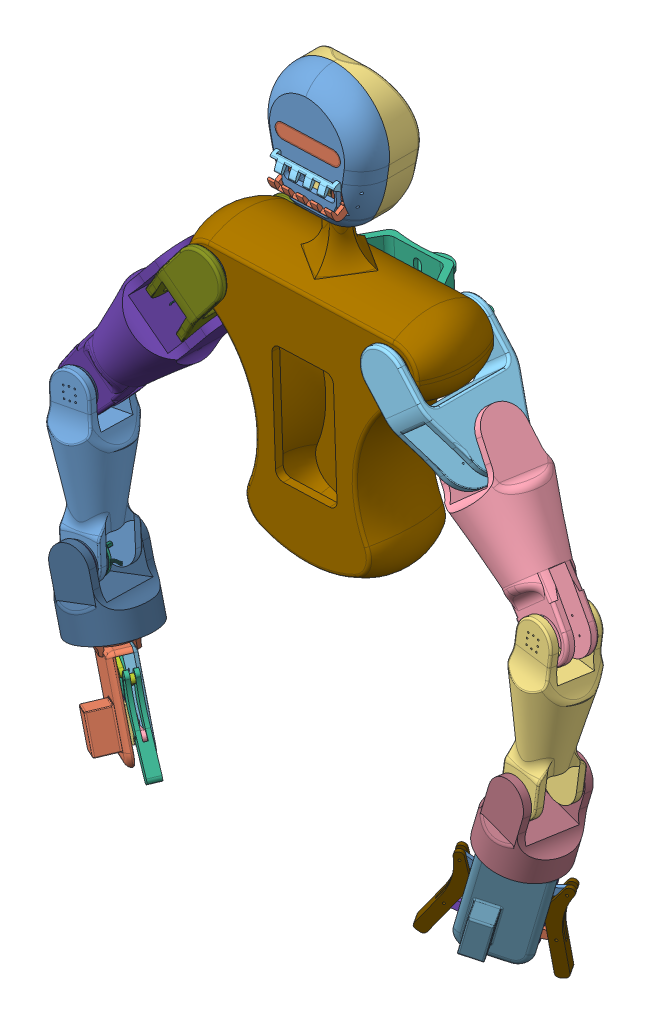
SolidWorks assembly assemblt jaloul main two, configuration Défaut. Lengths in mm.
Overall size (752.19 900.92 286).
290 component instances, 80 part files, 31 mates.
Components (placement in the parent):
- assembly head of jaloul-1: assembly head of jaloul [Défaut] at (50.4629 78.1935 73.0866) x (0.999385 0.035073 0) z (0 0 1) size (153.86 218.57 97.38)
  - head of jaloul-1: head of jaloul [Défaut] at (-2.8889 8.1989 56.9742) size (153.86 167.94 40.08)
  - RealSense_D435-1: RealSense_D435 [Default] at (-2 5.7058 43.2445) size (90.75 24.75 24.23)
  - ras jaloul men teli-1: ras jaloul men teli [Défaut] at (-4.3071 -4.0651 25.143) size (140.75 169.26 46.26)
  - raspberry-pi-5-sbc-simple.step-1: raspberry-pi-5-sbc-simple.step [Défaut] at (-2.8895 30.0633 18.143) size (90.56 58 19.2)
    - CSI_DSI-1.step-1: CSI_DSI-1.step [Défaut] at (-70.5 -36 11.75) size (3 15.5 4.1)
      - CSI_DSI_connector.step-1: CSI_DSI_connector.step [Défaut] at origin size (3 15.5 4.1)
    - CSI_DSI-2.step-1: CSI_DSI-2.step [Défaut] at (-70.5 -36 11.75) size (3 15.5 4.1)
      - CSI_DSI_connector.step-1: CSI_DSI_connector.step [Défaut] at (6.2 0 0) size (3 15.5 4.1)
    - pcba-components.step-1: pcba-components.step [Défaut] at (-70.5 -36 11.75) size (64.89 40.96 3.37)
      - pcba-components Geometry.step-1: pcba-components Geometry.step [Défaut] at origin size (62.02 39.27 3.37)
      - chips.step-1: chips.step [Défaut] at origin size (13.6 15 1)
    - poe.step-1: poe.step [Défaut] at (-70.5 -36 11.75) size (5.08 5.08 8.29)
      - poe Geometry.step-1: poe Geometry.step [Défaut] at origin size (5.08 5.08 1)
      - poe-pins.step-1: poe-pins.step [Défaut] at origin size (3.44 3.44 7.29)
    - usb-2-bank.step-1: usb-2-bank.step [Défaut] at (-0.7443 20 0.8) x (1 0 0) z (0 -1 0) size (17.07 15.5 13.76)
      - usb-2-bank Geometry.step-1: usb-2-bank Geometry.step [Défaut] at origin size (16.67 15.5 13.76)
      - usb2-port.step-1: usb2-port.step [Défaut] at origin size (4.42 5.12 12.5)
      - usb2-port.step-2: usb2-port.step [Défaut] at (0 -8.5 0) size (4.42 5.12 12.5)
    - usb-3-bank.step-1: usb-3-bank.step [Défaut] at (-0.5443 2.1 0.8) x (1 0 0) z (0 -1 0) size (17.07 15.5 13.76)
      - usb-3-bank Geometry.step-1: usb-3-bank Geometry.step [Défaut] at origin size (16.67 15.5 13.76)
      - usb3-port.step-1: usb3-port.step [Défaut] at origin size (4.42 5.12 12.5)
      - usb3-port.step-2: usb3-port.step [Défaut] at (0 -8.5 0) size (4.42 5.12 12.5)
    - connector.step-1: connector.step [Défaut] at (-70.5 -36 11.75) size (3 6 3.5)
    - ethernet.step-1: ethernet.step [Défaut] at (0 -35.55 0.8) x (1 0 0) z (0 -1 0) size (23.65 17.25 16)
    - gpio.step-1: gpio.step [Défaut] at (-70.53 -36.28 11.75) size (50.5 5 8.29)
    - hdmi-micro.step-1: hdmi-micro.step [Défaut] at (-0.3 0 0.8) x (1 0 0) z (0 -1 0) size (6.5 2.9 7.7)
    - hdmi-micro.step-2: hdmi-micro.step [Défaut] at (-13.8 0 0.8) x (1 0 0) z (0 -1 0) size (6.5 2.9 7.7)
    - IR.step-1: IR.step [Défaut] at (-70.5 -36 11.75) size (1.73 3.15 3.26)
    - mounting-holes.step-1: mounting-holes.step [Défaut] at (-70.5 -36 11.75) size (64 54.91 0.02)
    - pcb.step-1: pcb.step [Défaut] at (-70.5 -36 11.75) size (85 56 1.6)
    - pcie.step-1: pcie.step [Défaut] at (-70.5 -36 11.75) size (3 10.5 4.1)
    - pmic.step-1: pmic.step [Défaut] at (-70.5 -36 11.75) size (6 6 0.5)
    - pwr-connector.step-1: pwr-connector.step [Défaut] at (-70.5 -36 11.75) size (4 3 4.4)
    - rp1.step-1: rp1.step [Défaut] at (-70.5 -36 11.75) size (12 12 0.5)
    - sd-card.step-1: sd-card.step [Défaut] at (-70.5 -36 11.75) size (1.75 11.01 0.01) (hidden)
    - switch.step-1: switch.step [Défaut] at (-70.5 -36 11.75) size (3 4.75 1.77)
    - uart.step-1: uart.step [Défaut] at (-70.5 -36 11.75) size (5.25 3.25 4.4)
    - usb-c.step-1: usb-c.step [Défaut] at (-70.5 -36 11.75) size (9 7.5 3.2)
  - support head-1: support head [Défaut] at (-2.8895 -82.9367 30.143) x (0.544466 0 -0.838783) z (0 -1 0) size (62.95 62.95 55.38)
  - M90S_ali.step-1: M90S_ali.step [Défaut] at (23.3 -47.0367 54.243) x (0 -1 0) z (1 0 0) size (32.3 12.4 32.5)
    - axe.step-1: axe.step [Défaut] at origin size (4.9 4.9 14.2)
    - base001.step-1: base001.step [Défaut] at origin size (32.3 12.2 28.5)
    - etiquette.step-1: etiquette.step [Défaut] at origin size (20 0.2 10)
    - Tube.step-1: Tube.step [Défaut] at (5.4 0 -13.3) x (0 0 -1) z (1 0 0) size (1.2 1.2 3)
    - Cylindre.step-1: Cylindre.step [Défaut] at (5.4 0 -13.3) x (0 0 -1) z (1 0 0) size (0.4 0.4 4)
    - Tube001.step-1: Tube001.step [Défaut] at (5.4 -1.2 -13.3) x (0 0 -1) z (1 0 0) size (1.2 1.2 3)
    - Tube002.step-1: Tube002.step [Défaut] at (5.4 1.2 -13.3) x (0 0 -1) z (1 0 0) size (1.2 1.2 3)
    - etiquette001.step-1: etiquette001.step [Défaut] at (-10.8 0 0) x (-1 0 0) z (0 0 1) size (20 0.2 10)
    - Cylindre001.step-1: Cylindre001.step [Défaut] at (5.4 1.2 -13.3) x (0 0 -1) z (1 0 0) size (0.4 0.4 4)
    - Cylindre002.step-1: Cylindre002.step [Défaut] at (5.4 -1.2 -13.3) x (0 0 -1) z (1 0 0) size (0.4 0.4 4)
  - dents du jaloul-1: dents du jaloul [Défaut] at (-1.85 -55.3304 58.7391) x (-1 0 0) z (0 0.870081 0.492909) size (83 33.18 25.45)
  - MG90S_arm01.step-1: MG90S_arm01.step [Défaut] at (39.3 -47.0367 54.243) x (-1 0 0) z (0 0.870081 0.492909) size (4.8 21.4 6.8)
  - dent jaloul partie supérieur-1: dent jaloul partie supérieur [Défaut] at (-1.85 5.574 3.1017) size (83 33.18 25.45)
  - Symétriedents du jaloul-4: Symétriedents du jaloul [Défaut] at (-1.85 -21.043 58.7391) x (-1 0 0) z (0 0.870081 -0.492909) size (83 32.99 25.26)
- 4015 Motor.STEP-1: 4015 Motor.STEP [Défaut] at (-65.9697 -107.9474 135.4967) x (-0.675127 -0.737702 0) z (-0.737702 0.675127 0) size (63.54 36.6 63.54)
  - 4015定子.STEP-1: 4015定子.STEP [Défaut] at origin size (45.94 27.09 45.92)
  - MISUMI_C-E6800ZZ.STEP-1: MISUMI_C-E6800ZZ.STEP [Défaut] at (0 21.6 0) x (0 -1 0) z (-0.009932 0 0.999951) size (5 19 19)
  - MISUMI_C-E6800ZZ.STEP-2: MISUMI_C-E6800ZZ.STEP [Défaut] at (0 8 0) x (0 -1 0) z (-0.587995 0 0.808864) size (5 19 19)
  - 转子铝盖.STEP-1: 转子铝盖.STEP [Défaut] at (0 24 0) x (-0.665718 0 -0.746203) z (-0.746203 0 0.665718) size (45 23.5 45)
  - 磁钢片.STEP-1: 磁钢片.STEP [Défaut] at (5.7872 12.75 -20.8182) x (0.963466 0 0.267832) z (-0.267832 0 0.963466) size (4 16.5 1.3)
  - 中间不锈钢圈.STEP-1: 中间不锈钢圈.STEP [Défaut] at (0 4.5 0) x (0.999998 0 0.002002) z (0 1 0) size (45 45 16.5)
  - 磁钢片.STEP-2: 磁钢片.STEP [Défaut] at (-0.3124 12.75 -21.6054) x (0.999895 0 -0.014457) z (0.014457 0 0.999895) size (4 16.5 1.3)
  - 磁钢片.STEP-3: 磁钢片.STEP [Défaut] at (-6.3867 12.75 -20.6422) x (0.95532 0 -0.295574) z (0.295574 0 0.95532) size (4 16.5 1.3)
  - 磁钢片.STEP-4: 磁钢片.STEP [Défaut] at (-11.9435 12.75 -18.0067) x (0.83335 0 -0.552746) z (0.552746 0 0.83335) size (4 16.5 1.3)
  - 磁钢片.STEP-5: 磁钢片.STEP [Défaut] at (-16.5328 12.75 -13.9124) x (0.643867 0 -0.765138) z (0.765138 0 0.643867) size (4 16.5 1.3)
  - 磁钢片.STEP-6: 磁钢片.STEP [Défaut] at (-19.7827 12.75 -8.6911) x (0.402221 0 -0.915542) z (0.915542 0 0.402221) size (4 16.5 1.3)
  - 磁钢片.STEP-7: 磁钢片.STEP [Défaut] at (-21.4299 12.75 -2.7656) x (0.12799 0 -0.991775) z (0.991775 0 0.12799) size (4 16.5 1.3)
  - 磁钢片.STEP-8: 磁钢片.STEP [Défaut] at (-21.341 12.75 3.384) x (-0.15661 0 -0.987661) z (0.987661 0 -0.15661) size (4 16.5 1.3)
  - 磁钢片.STEP-9: 磁钢片.STEP [Défaut] at (-19.5232 12.75 9.2593) x (-0.428522 0 -0.903531) z (0.903531 0 -0.428522) size (4 16.5 1.3)
  - 磁钢片.STEP-10: 磁钢片.STEP [Défaut] at (-16.1237 12.75 14.3846) x (-0.665718 0 -0.746203) z (0.746203 0 -0.665718) size (4 16.5 1.3)
  - 磁钢片.STEP-11: 磁钢片.STEP [Défaut] at (-11.418 12.75 18.3445) x (-0.848982 0 -0.528423) z (0.528423 0 -0.848982) size (4 16.5 1.3)
  - 磁钢片.STEP-12: 磁钢片.STEP [Défaut] at (-5.7872 12.75 20.8182) x (-0.963466 0 -0.267832) z (0.267832 0 -0.963466) size (4 16.5 1.3)
  - 磁钢片.STEP-13: 磁钢片.STEP [Défaut] at (0.3124 12.75 21.6054) x (-0.999895 0 0.014457) z (-0.014457 0 -0.999895) size (4 16.5 1.3)
  - 磁钢片.STEP-14: 磁钢片.STEP [Défaut] at (6.3867 12.75 20.6422) x (-0.95532 0 0.295574) z (-0.295574 0 -0.95532) size (4 16.5 1.3)
  - 磁钢片.STEP-15: 磁钢片.STEP [Défaut] at (11.9435 12.75 18.0067) x (-0.83335 0 0.552746) z (-0.552746 0 -0.83335) size (4 16.5 1.3)
  - 磁钢片.STEP-16: 磁钢片.STEP [Défaut] at (16.5328 12.75 13.9124) x (-0.643867 0 0.765138) z (-0.765138 0 -0.643867) size (4 16.5 1.3)
  - 磁钢片.STEP-17: 磁钢片.STEP [Défaut] at (19.7827 12.75 8.6911) x (-0.402221 0 0.915542) z (-0.915542 0 -0.402221) size (4 16.5 1.3)
  - 磁钢片.STEP-18: 磁钢片.STEP [Défaut] at (21.4299 12.75 2.7656) x (-0.12799 0 0.991775) z (-0.991775 0 -0.12799) size (4 16.5 1.3)
  - 磁钢片.STEP-19: 磁钢片.STEP [Défaut] at (21.341 12.75 -3.384) x (0.15661 0 0.987661) z (-0.987661 0 0.15661) size (4 16.5 1.3)
  - 磁钢片.STEP-20: 磁钢片.STEP [Défaut] at (19.5232 12.75 -9.2593) x (0.428522 0 0.903531) z (-0.903531 0 0.428522) size (4 16.5 1.3)
  - 磁钢片.STEP-21: 磁钢片.STEP [Défaut] at (16.1237 12.75 -14.3846) x (0.665718 0 0.746203) z (-0.746203 0 0.665718) size (4 16.5 1.3)
  - 磁钢片.STEP-22: 磁钢片.STEP [Défaut] at (11.418 12.75 -18.3445) x (0.848982 0 0.528423) z (-0.528423 0 0.848982) size (4 16.5 1.3)
  - 径向磁环.STEP-1: 径向磁环.STEP [Défaut] at (0 0.5 0) x (0.972164 0 0.234302) z (0 -1 0) size (10 10 2.5)
  - 径向磁环固定环.STEP-1: 径向磁环固定环.STEP [Défaut] at (0 -2 0) x (0.933781 0 0.357846) z (0 1 0) size (11.2 12.93 5)
  - 铜柱M2.5x4+4.STEP-1: 铜柱M2.5x4+4.STEP [Défaut] at (14 -4 0) size (5 8 5.77)
  - 铜柱M2.5x4+4.STEP-2: 铜柱M2.5x4+4.STEP [Défaut] at (0 -4 -14) x (0.982082 0 -0.188455) z (0.188455 0 0.982082) size (5 8 5.77)
  - 铜柱M2.5x4+4.STEP-3: 铜柱M2.5x4+4.STEP [Défaut] at (0 -4 14) x (0.918365 0 -0.395734) z (0.395734 0 0.918365) size (5 8 5.77)
  - 铜柱M2.5x4+4.STEP-4: 铜柱M2.5x4+4.STEP [Défaut] at (-14 -4 0) x (0.8 0 -0.6) z (0.6 0 0.8) size (5 8 5.77)
  - AS5600磁编码器-圆.STEP-1: AS5600磁编码器-圆.STEP [Défaut] at (-0.3592 -5.6 0) x (0.707107 0 -0.707107) z (0 1 0) size (31.97 31.97 7.67)
  - 铜柱M2.5x7+4.STEP-1: 铜柱M2.5x7+4.STEP [Défaut] at (0 -12.6 -14) x (0.898383 0 -0.439214) z (0.439214 0 0.898383) size (5 11 5.77)
  - 铜柱M2.5x7+4.STEP-2: 铜柱M2.5x7+4.STEP [Défaut] at (-14 -12.6 0) x (0.799513 0 -0.600648) z (0.600648 0 0.799513) size (5 11 5.77)
  - 铜柱M2.5x7+4.STEP-3: 铜柱M2.5x7+4.STEP [Défaut] at (14 -12.6 0) x (0.651231 0 -0.758879) z (0.758879 0 0.651231) size (5 11 5.77)
  - 铜柱M2.5x7+4.STEP-4: 铜柱M2.5x7+4.STEP [Défaut] at (0 -12.6 14) x (0.455178 0 -0.890401) z (0.890401 0 0.455178) size (5 11 5.77)
- link 1 JALOUL-1: link 1 JALOUL [Défaut] at (-74.3576 -118.8426 159.4967) x (0.61003 0.792378 0) z (0 0 1) size (167.5 60.6 125)
- 4015 Motor.STEP-2: 4015 Motor.STEP [Défaut] at (-134.1638 -178.494 106.9967) x (0.604333 0.784978 0.136349) z (-0.083177 -0.10804 0.990661) size (63.54 36.6 63.54)
  - 4015定子.STEP-1: 4015定子.STEP [Défaut] at origin size (45.94 27.09 45.92)
  - MISUMI_C-E6800ZZ.STEP-1: MISUMI_C-E6800ZZ.STEP [Défaut] at (0 21.6 0) x (0 -1 0) z (-0.009932 0 0.999951) size (5 19 19)
  - MISUMI_C-E6800ZZ.STEP-2: MISUMI_C-E6800ZZ.STEP [Défaut] at (0 8 0) x (0 -1 0) z (-0.587995 0 0.808864) size (5 19 19)
  - 转子铝盖.STEP-1: 转子铝盖.STEP [Défaut] at (0 24 0) x (-0.665718 0 -0.746203) z (-0.746203 0 0.665718) size (45 23.5 45)
  - 磁钢片.STEP-1: 磁钢片.STEP [Défaut] at (5.7872 12.75 -20.8182) x (0.963466 0 0.267832) z (-0.267832 0 0.963466) size (4 16.5 1.3)
  - 中间不锈钢圈.STEP-1: 中间不锈钢圈.STEP [Défaut] at (0 4.5 0) x (0.999998 0 0.002002) z (0 1 0) size (45 45 16.5)
  - 磁钢片.STEP-2: 磁钢片.STEP [Défaut] at (-0.3124 12.75 -21.6054) x (0.999895 0 -0.014457) z (0.014457 0 0.999895) size (4 16.5 1.3)
  - 磁钢片.STEP-3: 磁钢片.STEP [Défaut] at (-6.3867 12.75 -20.6422) x (0.95532 0 -0.295574) z (0.295574 0 0.95532) size (4 16.5 1.3)
  - 磁钢片.STEP-4: 磁钢片.STEP [Défaut] at (-11.9435 12.75 -18.0067) x (0.83335 0 -0.552746) z (0.552746 0 0.83335) size (4 16.5 1.3)
  - 磁钢片.STEP-5: 磁钢片.STEP [Défaut] at (-16.5328 12.75 -13.9124) x (0.643867 0 -0.765138) z (0.765138 0 0.643867) size (4 16.5 1.3)
  - 磁钢片.STEP-6: 磁钢片.STEP [Défaut] at (-19.7827 12.75 -8.6911) x (0.402221 0 -0.915542) z (0.915542 0 0.402221) size (4 16.5 1.3)
  - 磁钢片.STEP-7: 磁钢片.STEP [Défaut] at (-21.4299 12.75 -2.7656) x (0.12799 0 -0.991775) z (0.991775 0 0.12799) size (4 16.5 1.3)
  - 磁钢片.STEP-8: 磁钢片.STEP [Défaut] at (-21.341 12.75 3.384) x (-0.15661 0 -0.987661) z (0.987661 0 -0.15661) size (4 16.5 1.3)
  - 磁钢片.STEP-9: 磁钢片.STEP [Défaut] at (-19.5232 12.75 9.2593) x (-0.428522 0 -0.903531) z (0.903531 0 -0.428522) size (4 16.5 1.3)
  - 磁钢片.STEP-10: 磁钢片.STEP [Défaut] at (-16.1237 12.75 14.3846) x (-0.665718 0 -0.746203) z (0.746203 0 -0.665718) size (4 16.5 1.3)
  - 磁钢片.STEP-11: 磁钢片.STEP [Défaut] at (-11.418 12.75 18.3445) x (-0.848982 0 -0.528423) z (0.528423 0 -0.848982) size (4 16.5 1.3)
  - 磁钢片.STEP-12: 磁钢片.STEP [Défaut] at (-5.7872 12.75 20.8182) x (-0.963466 0 -0.267832) z (0.267832 0 -0.963466) size (4 16.5 1.3)
  - 磁钢片.STEP-13: 磁钢片.STEP [Défaut] at (0.3124 12.75 21.6054) x (-0.999895 0 0.014457) z (-0.014457 0 -0.999895) size (4 16.5 1.3)
  - 磁钢片.STEP-14: 磁钢片.STEP [Défaut] at (6.3867 12.75 20.6422) x (-0.95532 0 0.295574) z (-0.295574 0 -0.95532) size (4 16.5 1.3)
  - 磁钢片.STEP-15: 磁钢片.STEP [Défaut] at (11.9435 12.75 18.0067) x (-0.83335 0 0.552746) z (-0.552746 0 -0.83335) size (4 16.5 1.3)
  - 磁钢片.STEP-16: 磁钢片.STEP [Défaut] at (16.5328 12.75 13.9124) x (-0.643867 0 0.765138) z (-0.765138 0 -0.643867) size (4 16.5 1.3)
  - 磁钢片.STEP-17: 磁钢片.STEP [Défaut] at (19.7827 12.75 8.6911) x (-0.402221 0 0.915542) z (-0.915542 0 -0.402221) size (4 16.5 1.3)
  - 磁钢片.STEP-18: 磁钢片.STEP [Défaut] at (21.4299 12.75 2.7656) x (-0.12799 0 0.991775) z (-0.991775 0 -0.12799) size (4 16.5 1.3)
  - 磁钢片.STEP-19: 磁钢片.STEP [Défaut] at (21.341 12.75 -3.384) x (0.15661 0 0.987661) z (-0.987661 0 0.15661) size (4 16.5 1.3)
  - 磁钢片.STEP-20: 磁钢片.STEP [Défaut] at (19.5232 12.75 -9.2593) x (0.428522 0 0.903531) z (-0.903531 0 0.428522) size (4 16.5 1.3)
  - 磁钢片.STEP-21: 磁钢片.STEP [Défaut] at (16.1237 12.75 -14.3846) x (0.665718 0 0.746203) z (-0.746203 0 0.665718) size (4 16.5 1.3)
  - 磁钢片.STEP-22: 磁钢片.STEP [Défaut] at (11.418 12.75 -18.3445) x (0.848982 0 0.528423) z (-0.528423 0 0.848982) size (4 16.5 1.3)
  - 径向磁环.STEP-1: 径向磁环.STEP [Défaut] at (0 0.5 0) x (0.972164 0 0.234302) z (0 -1 0) size (10 10 2.5)
  - 径向磁环固定环.STEP-1: 径向磁环固定环.STEP [Défaut] at (0 -2 0) x (0.933781 0 0.357846) z (0 1 0) size (11.2 12.93 5)
  - 铜柱M2.5x4+4.STEP-1: 铜柱M2.5x4+4.STEP [Défaut] at (14 -4 0) size (5 8 5.77)
  - 铜柱M2.5x4+4.STEP-2: 铜柱M2.5x4+4.STEP [Défaut] at (0 -4 -14) x (0.982082 0 -0.188455) z (0.188455 0 0.982082) size (5 8 5.77)
  - 铜柱M2.5x4+4.STEP-3: 铜柱M2.5x4+4.STEP [Défaut] at (0 -4 14) x (0.918365 0 -0.395734) z (0.395734 0 0.918365) size (5 8 5.77)
  - 铜柱M2.5x4+4.STEP-4: 铜柱M2.5x4+4.STEP [Défaut] at (-14 -4 0) x (0.8 0 -0.6) z (0.6 0 0.8) size (5 8 5.77)
  - AS5600磁编码器-圆.STEP-1: AS5600磁编码器-圆.STEP [Défaut] at (-0.3592 -5.6 0) x (0.707107 0 -0.707107) z (0 1 0) size (31.97 31.97 7.67)
  - 铜柱M2.5x7+4.STEP-1: 铜柱M2.5x7+4.STEP [Défaut] at (0 -12.6 -14) x (0.898383 0 -0.439214) z (0.439214 0 0.898383) size (5 11 5.77)
  - 铜柱M2.5x7+4.STEP-2: 铜柱M2.5x7+4.STEP [Défaut] at (-14 -12.6 0) x (0.799513 0 -0.600648) z (0.600648 0 0.799513) size (5 11 5.77)
  - 铜柱M2.5x7+4.STEP-3: 铜柱M2.5x7+4.STEP [Défaut] at (14 -12.6 0) x (0.651231 0 -0.758879) z (0.758879 0 0.651231) size (5 11 5.77)
  - 铜柱M2.5x7+4.STEP-4: 铜柱M2.5x7+4.STEP [Défaut] at (0 -12.6 14) x (0.455178 0 -0.890401) z (0.890401 0 0.455178) size (5 11 5.77)
- link 2 JALOUL-1: link 2 JALOUL [Défaut] at (-194.9505 -201.7159 82.9556) x (0.606326 0.787567 -0.110033) z (0.067124 0.087188 0.993928) size (247.23 121.75 118.52)
- 4015 Motor.STEP-3: 4015 Motor.STEP [Défaut] at (-242.3982 -333.0153 128.8669) x (-0.985892 -0.147294 0.079502) z (-0.153331 0.985242 -0.076071) size (63.54 36.6 63.54)
  - 4015定子.STEP-1: 4015定子.STEP [Défaut] at origin size (45.94 27.09 45.92)
  - MISUMI_C-E6800ZZ.STEP-1: MISUMI_C-E6800ZZ.STEP [Défaut] at (0 21.6 0) x (0 -1 0) z (-0.009932 0 0.999951) size (5 19 19)
  - MISUMI_C-E6800ZZ.STEP-2: MISUMI_C-E6800ZZ.STEP [Défaut] at (0 8 0) x (0 -1 0) z (-0.587995 0 0.808864) size (5 19 19)
  - 转子铝盖.STEP-1: 转子铝盖.STEP [Défaut] at (0 24 0) x (-0.665718 0 -0.746203) z (-0.746203 0 0.665718) size (45 23.5 45)
  - 磁钢片.STEP-1: 磁钢片.STEP [Défaut] at (5.7872 12.75 -20.8182) x (0.963466 0 0.267832) z (-0.267832 0 0.963466) size (4 16.5 1.3)
  - 中间不锈钢圈.STEP-1: 中间不锈钢圈.STEP [Défaut] at (0 4.5 0) x (0.999998 0 0.002002) z (0 1 0) size (45 45 16.5)
  - 磁钢片.STEP-2: 磁钢片.STEP [Défaut] at (-0.3124 12.75 -21.6054) x (0.999895 0 -0.014457) z (0.014457 0 0.999895) size (4 16.5 1.3)
  - 磁钢片.STEP-3: 磁钢片.STEP [Défaut] at (-6.3867 12.75 -20.6422) x (0.95532 0 -0.295574) z (0.295574 0 0.95532) size (4 16.5 1.3)
  - 磁钢片.STEP-4: 磁钢片.STEP [Défaut] at (-11.9435 12.75 -18.0067) x (0.83335 0 -0.552746) z (0.552746 0 0.83335) size (4 16.5 1.3)
  - 磁钢片.STEP-5: 磁钢片.STEP [Défaut] at (-16.5328 12.75 -13.9124) x (0.643867 0 -0.765138) z (0.765138 0 0.643867) size (4 16.5 1.3)
  - 磁钢片.STEP-6: 磁钢片.STEP [Défaut] at (-19.7827 12.75 -8.6911) x (0.402221 0 -0.915542) z (0.915542 0 0.402221) size (4 16.5 1.3)
  - 磁钢片.STEP-7: 磁钢片.STEP [Défaut] at (-21.4299 12.75 -2.7656) x (0.12799 0 -0.991775) z (0.991775 0 0.12799) size (4 16.5 1.3)
  - 磁钢片.STEP-8: 磁钢片.STEP [Défaut] at (-21.341 12.75 3.384) x (-0.15661 0 -0.987661) z (0.987661 0 -0.15661) size (4 16.5 1.3)
  - 磁钢片.STEP-9: 磁钢片.STEP [Défaut] at (-19.5232 12.75 9.2593) x (-0.428522 0 -0.903531) z (0.903531 0 -0.428522) size (4 16.5 1.3)
  - 磁钢片.STEP-10: 磁钢片.STEP [Défaut] at (-16.1237 12.75 14.3846) x (-0.665718 0 -0.746203) z (0.746203 0 -0.665718) size (4 16.5 1.3)
  - 磁钢片.STEP-11: 磁钢片.STEP [Défaut] at (-11.418 12.75 18.3445) x (-0.848982 0 -0.528423) z (0.528423 0 -0.848982) size (4 16.5 1.3)
  - 磁钢片.STEP-12: 磁钢片.STEP [Défaut] at (-5.7872 12.75 20.8182) x (-0.963466 0 -0.267832) z (0.267832 0 -0.963466) size (4 16.5 1.3)
  - 磁钢片.STEP-13: 磁钢片.STEP [Défaut] at (0.3124 12.75 21.6054) x (-0.999895 0 0.014457) z (-0.014457 0 -0.999895) size (4 16.5 1.3)
  - 磁钢片.STEP-14: 磁钢片.STEP [Défaut] at (6.3867 12.75 20.6422) x (-0.95532 0 0.295574) z (-0.295574 0 -0.95532) size (4 16.5 1.3)
  - 磁钢片.STEP-15: 磁钢片.STEP [Défaut] at (11.9435 12.75 18.0067) x (-0.83335 0 0.552746) z (-0.552746 0 -0.83335) size (4 16.5 1.3)
  - 磁钢片.STEP-16: 磁钢片.STEP [Défaut] at (16.5328 12.75 13.9124) x (-0.643867 0 0.765138) z (-0.765138 0 -0.643867) size (4 16.5 1.3)
  - 磁钢片.STEP-17: 磁钢片.STEP [Défaut] at (19.7827 12.75 8.6911) x (-0.402221 0 0.915542) z (-0.915542 0 -0.402221) size (4 16.5 1.3)
  - 磁钢片.STEP-18: 磁钢片.STEP [Défaut] at (21.4299 12.75 2.7656) x (-0.12799 0 0.991775) z (-0.991775 0 -0.12799) size (4 16.5 1.3)
  - 磁钢片.STEP-19: 磁钢片.STEP [Défaut] at (21.341 12.75 -3.384) x (0.15661 0 0.987661) z (-0.987661 0 0.15661) size (4 16.5 1.3)
  - 磁钢片.STEP-20: 磁钢片.STEP [Défaut] at (19.5232 12.75 -9.2593) x (0.428522 0 0.903531) z (-0.903531 0 0.428522) size (4 16.5 1.3)
  - 磁钢片.STEP-21: 磁钢片.STEP [Défaut] at (16.1237 12.75 -14.3846) x (0.665718 0 0.746203) z (-0.746203 0 0.665718) size (4 16.5 1.3)
  - 磁钢片.STEP-22: 磁钢片.STEP [Défaut] at (11.418 12.75 -18.3445) x (0.848982 0 0.528423) z (-0.528423 0 0.848982) size (4 16.5 1.3)
  - 径向磁环.STEP-1: 径向磁环.STEP [Défaut] at (0 0.5 0) x (0.972164 0 0.234302) z (0 -1 0) size (10 10 2.5)
  - 径向磁环固定环.STEP-1: 径向磁环固定环.STEP [Défaut] at (0 -2 0) x (0.933781 0 0.357846) z (0 1 0) size (11.2 12.93 5)
  - 铜柱M2.5x4+4.STEP-1: 铜柱M2.5x4+4.STEP [Défaut] at (14 -4 0) size (5 8 5.77)
  - 铜柱M2.5x4+4.STEP-2: 铜柱M2.5x4+4.STEP [Défaut] at (0 -4 -14) x (0.982082 0 -0.188455) z (0.188455 0 0.982082) size (5 8 5.77)
  - 铜柱M2.5x4+4.STEP-3: 铜柱M2.5x4+4.STEP [Défaut] at (0 -4 14) x (0.918365 0 -0.395734) z (0.395734 0 0.918365) size (5 8 5.77)
  - 铜柱M2.5x4+4.STEP-4: 铜柱M2.5x4+4.STEP [Défaut] at (-14 -4 0) x (0.8 0 -0.6) z (0.6 0 0.8) size (5 8 5.77)
  - AS5600磁编码器-圆.STEP-1: AS5600磁编码器-圆.STEP [Défaut] at (-0.3592 -5.6 0) x (0.707107 0 -0.707107) z (0 1 0) size (31.97 31.97 7.67)
  - 铜柱M2.5x7+4.STEP-1: 铜柱M2.5x7+4.STEP [Défaut] at (0 -12.6 -14) x (0.898383 0 -0.439214) z (0.439214 0 0.898383) size (5 11 5.77)
  - 铜柱M2.5x7+4.STEP-2: 铜柱M2.5x7+4.STEP [Défaut] at (-14 -12.6 0) x (0.799513 0 -0.600648) z (0.600648 0 0.799513) size (5 11 5.77)
  - 铜柱M2.5x7+4.STEP-3: 铜柱M2.5x7+4.STEP [Défaut] at (14 -12.6 0) x (0.651231 0 -0.758879) z (0.758879 0 0.651231) size (5 11 5.77)
  - 铜柱M2.5x7+4.STEP-4: 铜柱M2.5x7+4.STEP [Défaut] at (0 -12.6 14) x (0.455178 0 -0.890401) z (0.890401 0 0.455178) size (5 11 5.77)
- ISO 15 RBB - 105 - 8,SI,NC,8_68-1: ISO 15 RBB - 105 - 8,SI,NC,8_68 [ISO 15 RBB - 105 - 8,SI,NC,8_68] at (-316.6056 -16.061 376.3383) x (0.875338 0.056415 0.480209) z (0.163001 -0.969462 -0.18323) size (5 14 14) (hidden)
- ISO 15 RBB - 105 - 8,SI,NC,8_68-2: ISO 15 RBB - 105 - 8,SI,NC,8_68 [ISO 15 RBB - 105 - 8,SI,NC,8_68] at (-108.995 -208.9135 106.9967) x (0.792378 -0.61003 0) z (0 0 1) size (5 14 14)
- LINK 3 JALOUL-1: LINK 3 JALOUL [Défaut] at (-257.529 -387.5668 168.8818) x (-0.13288 0.988082 -0.077701) z (0.988857 0.126858 -0.077909) size (224.5 90.56 90.03)
- 4015 Motor.STEP-5: 4015 Motor.STEP [Défaut] at (-218.4729 -505.0577 152.4039) x (-0.746862 0.664932 -0.00789) z (0.661582 0.741798 -0.10975) size (63.54 36.6 63.54)
  - 4015定子.STEP-1: 4015定子.STEP [Défaut] at origin size (45.94 27.09 45.92)
  - MISUMI_C-E6800ZZ.STEP-1: MISUMI_C-E6800ZZ.STEP [Défaut] at (0 21.6 0) x (0 -1 0) z (-0.009932 0 0.999951) size (5 19 19)
  - MISUMI_C-E6800ZZ.STEP-2: MISUMI_C-E6800ZZ.STEP [Défaut] at (0 8 0) x (0 -1 0) z (-0.587995 0 0.808864) size (5 19 19)
  - 转子铝盖.STEP-1: 转子铝盖.STEP [Défaut] at (0 24 0) x (-0.665718 0 -0.746203) z (-0.746203 0 0.665718) size (45 23.5 45)
  - 磁钢片.STEP-1: 磁钢片.STEP [Défaut] at (5.7872 12.75 -20.8182) x (0.963466 0 0.267832) z (-0.267832 0 0.963466) size (4 16.5 1.3)
  - 中间不锈钢圈.STEP-1: 中间不锈钢圈.STEP [Défaut] at (0 4.5 0) x (0.999998 0 0.002002) z (0 1 0) size (45 45 16.5)
  - 磁钢片.STEP-2: 磁钢片.STEP [Défaut] at (-0.3124 12.75 -21.6054) x (0.999895 0 -0.014457) z (0.014457 0 0.999895) size (4 16.5 1.3)
  - 磁钢片.STEP-3: 磁钢片.STEP [Défaut] at (-6.3867 12.75 -20.6422) x (0.95532 0 -0.295574) z (0.295574 0 0.95532) size (4 16.5 1.3)
  - 磁钢片.STEP-4: 磁钢片.STEP [Défaut] at (-11.9435 12.75 -18.0067) x (0.83335 0 -0.552746) z (0.552746 0 0.83335) size (4 16.5 1.3)
  - 磁钢片.STEP-5: 磁钢片.STEP [Défaut] at (-16.5328 12.75 -13.9124) x (0.643867 0 -0.765138) z (0.765138 0 0.643867) size (4 16.5 1.3)
  - 磁钢片.STEP-6: 磁钢片.STEP [Défaut] at (-19.7827 12.75 -8.6911) x (0.402221 0 -0.915542) z (0.915542 0 0.402221) size (4 16.5 1.3)
  - 磁钢片.STEP-7: 磁钢片.STEP [Défaut] at (-21.4299 12.75 -2.7656) x (0.12799 0 -0.991775) z (0.991775 0 0.12799) size (4 16.5 1.3)
  - 磁钢片.STEP-8: 磁钢片.STEP [Défaut] at (-21.341 12.75 3.384) x (-0.15661 0 -0.987661) z (0.987661 0 -0.15661) size (4 16.5 1.3)
  - 磁钢片.STEP-9: 磁钢片.STEP [Défaut] at (-19.5232 12.75 9.2593) x (-0.428522 0 -0.903531) z (0.903531 0 -0.428522) size (4 16.5 1.3)
  - 磁钢片.STEP-10: 磁钢片.STEP [Défaut] at (-16.1237 12.75 14.3846) x (-0.665718 0 -0.746203) z (0.746203 0 -0.665718) size (4 16.5 1.3)
  - 磁钢片.STEP-11: 磁钢片.STEP [Défaut] at (-11.418 12.75 18.3445) x (-0.848982 0 -0.528423) z (0.528423 0 -0.848982) size (4 16.5 1.3)
  - 磁钢片.STEP-12: 磁钢片.STEP [Défaut] at (-5.7872 12.75 20.8182) x (-0.963466 0 -0.267832) z (0.267832 0 -0.963466) size (4 16.5 1.3)
  - 磁钢片.STEP-13: 磁钢片.STEP [Défaut] at (0.3124 12.75 21.6054) x (-0.999895 0 0.014457) z (-0.014457 0 -0.999895) size (4 16.5 1.3)
  - 磁钢片.STEP-14: 磁钢片.STEP [Défaut] at (6.3867 12.75 20.6422) x (-0.95532 0 0.295574) z (-0.295574 0 -0.95532) size (4 16.5 1.3)
  - 磁钢片.STEP-15: 磁钢片.STEP [Défaut] at (11.9435 12.75 18.0067) x (-0.83335 0 0.552746) z (-0.552746 0 -0.83335) size (4 16.5 1.3)
  - 磁钢片.STEP-16: 磁钢片.STEP [Défaut] at (16.5328 12.75 13.9124) x (-0.643867 0 0.765138) z (-0.765138 0 -0.643867) size (4 16.5 1.3)
  - 磁钢片.STEP-17: 磁钢片.STEP [Défaut] at (19.7827 12.75 8.6911) x (-0.402221 0 0.915542) z (-0.915542 0 -0.402221) size (4 16.5 1.3)
  - 磁钢片.STEP-18: 磁钢片.STEP [Défaut] at (21.4299 12.75 2.7656) x (-0.12799 0 0.991775) z (-0.991775 0 -0.12799) size (4 16.5 1.3)
  - 磁钢片.STEP-19: 磁钢片.STEP [Défaut] at (21.341 12.75 -3.384) x (0.15661 0 0.987661) z (-0.987661 0 0.15661) size (4 16.5 1.3)
  - 磁钢片.STEP-20: 磁钢片.STEP [Défaut] at (19.5232 12.75 -9.2593) x (0.428522 0 0.903531) z (-0.903531 0 0.428522) size (4 16.5 1.3)
  - 磁钢片.STEP-21: 磁钢片.STEP [Défaut] at (16.1237 12.75 -14.3846) x (0.665718 0 0.746203) z (-0.746203 0 0.665718) size (4 16.5 1.3)
  - 磁钢片.STEP-22: 磁钢片.STEP [Défaut] at (11.418 12.75 -18.3445) x (0.848982 0 0.528423) z (-0.528423 0 0.848982) size (4 16.5 1.3)
  - 径向磁环.STEP-1: 径向磁环.STEP [Défaut] at (0 0.5 0) x (0.972164 0 0.234302) z (0 -1 0) size (10 10 2.5)
  - 径向磁环固定环.STEP-1: 径向磁环固定环.STEP [Défaut] at (0 -2 0) x (0.933781 0 0.357846) z (0 1 0) size (11.2 12.93 5)
  - 铜柱M2.5x4+4.STEP-1: 铜柱M2.5x4+4.STEP [Défaut] at (14 -4 0) size (5 8 5.77)
  - 铜柱M2.5x4+4.STEP-2: 铜柱M2.5x4+4.STEP [Défaut] at (0 -4 -14) x (0.982082 0 -0.188455) z (0.188455 0 0.982082) size (5 8 5.77)
  - 铜柱M2.5x4+4.STEP-3: 铜柱M2.5x4+4.STEP [Défaut] at (0 -4 14) x (0.918365 0 -0.395734) z (0.395734 0 0.918365) size (5 8 5.77)
  - 铜柱M2.5x4+4.STEP-4: 铜柱M2.5x4+4.STEP [Défaut] at (-14 -4 0) x (0.8 0 -0.6) z (0.6 0 0.8) size (5 8 5.77)
  - AS5600磁编码器-圆.STEP-1: AS5600磁编码器-圆.STEP [Défaut] at (-0.3592 -5.6 0) x (0.707107 0 -0.707107) z (0 1 0) size (31.97 31.97 7.67)
  - 铜柱M2.5x7+4.STEP-1: 铜柱M2.5x7+4.STEP [Défaut] at (0 -12.6 -14) x (0.898383 0 -0.439214) z (0.439214 0 0.898383) size (5 11 5.77)
  - 铜柱M2.5x7+4.STEP-2: 铜柱M2.5x7+4.STEP [Défaut] at (-14 -12.6 0) x (0.799513 0 -0.600648) z (0.600648 0 0.799513) size (5 11 5.77)
  - 铜柱M2.5x7+4.STEP-3: 铜柱M2.5x7+4.STEP [Défaut] at (14 -12.6 0) x (0.651231 0 -0.758879) z (0.758879 0 0.651231) size (5 11 5.77)
  - 铜柱M2.5x7+4.STEP-4: 铜柱M2.5x7+4.STEP [Défaut] at (0 -12.6 14) x (0.455178 0 -0.890401) z (0.890401 0 0.455178) size (5 11 5.77)
- assembly gripper  jalloul-1: assembly gripper  jalloul [Défaut] at (-235.5373 -657.7977 251.6936) x (0.796305 0.294379 0.528431) z (0.51977 0.113862 -0.846685) size (200.08 125.27 59)
  - BASE GRIPPER JALLOUL-1: BASE GRIPPER JALLOUL [Défaut] at (0.9473 -0.842 100) size (80.77 119.68 54)
  - servo Assem-1: servo Assem [Default] at (59.4312 -11.8514 114.1715) x (-1 0 0) z (0 1 0) size (20 45 54)
    - servo strong junk 2-2: servo strong junk 2 [Default] at (33.4839 -39.4715 49.0094) size (20 45 54)
  - pignon jlayla-2: pignon jlayla [ISO - Spur gear 2.25M 14T 20PA 5FW ---S14A75H50L5.0N] at (15.9473 27.158 120.7) x (0 0 -1) z (-0.171995 -0.985098 0) size (5 63.26 36)
  - entretoise gripper JALLOUL-1: entretoise gripper JALLOUL [Défaut] at (20.9473 -45.842 105) x (0.938027 -0.346563 0) z (0 0 1) size (5.07 5.86 35) (hidden)
  - entretoise gripper JALLOUL-2: entretoise gripper JALLOUL [Défaut] at (-19.0527 -45.842 104.8272) x (0.101066 -0.99488 0) z (0 0 1) size (5.07 5.86 35) (hidden)
  - gripper jaloul partie inférieur chg2-1: gripper jaloul partie inférieur chg2 [Défaut] at (0.9473 -0.842 125.7) size (80.01 120 5.01)
  - yed jaloul-1: yed jaloul [Défaut] at (35.4301 -10.2294 110.7) x (0.933099 -0.359619 0) z (0 0 1) size (39.43 112.05 15.1)
  - guidage YED JALLOUL-1: guidage YED JALLOUL [Défaut] at (34.4721 -28.3808 115.7) x (0.926239 -0.376938 0) z (0 0 1) size (50 10 5)
  - Symétriepignon jlayla-3: Symétriepignon jlayla [ISO - Spur gear 2.25M 14T 20PA 5FW ---S14A75H50L5.0N] at (-14.0527 27.158 120.7) x (0 0 -1) z (-0.171995 0.985098 0) size (5 63.26 36)
  - yed jaloul-2: yed jaloul [Défaut] at (-33.5355 -10.2294 125.7) x (-0.933099 -0.359619 0) z (0 0 -1) size (39.43 112.05 15.1)
  - guidage YED JALLOUL-2: guidage YED JALLOUL [Défaut] at (-32.5775 -28.3808 115.7) x (0.926239 0.376938 0) z (0 0 1) size (50 10 5)
- body of the robot-1: body of the robot [Défaut] at (52.9043 -73.7572 144.4967) x (0.999385 0.035073 0) z (0 0 1) size (328.01 328.01 100)
- link 4-1: link 4 [Défaut] at (-225.981 -552.3767 191.2696) x (-0.067124 -0.087188 -0.993928) z (0.948555 0.303351 -0.09067) size (98.62 100 98.62)
- 4015 Motor.STEP-7: 4015 Motor.STEP [Défaut] at (-201.7163 -558.9362 147.4466) x (-0.127352 -0.106316 -0.986143) z (-0.942361 -0.297187 0.153738) size (63.54 36.6 63.54)
  - 4015定子.STEP-1: 4015定子.STEP [Défaut] at origin size (45.94 27.09 45.92)
  - MISUMI_C-E6800ZZ.STEP-1: MISUMI_C-E6800ZZ.STEP [Défaut] at (0 21.6 0) x (0 -1 0) z (-0.009932 0 0.999951) size (5 19 19)
  - MISUMI_C-E6800ZZ.STEP-2: MISUMI_C-E6800ZZ.STEP [Défaut] at (0 8 0) x (0 -1 0) z (-0.587995 0 0.808864) size (5 19 19)
  - 转子铝盖.STEP-1: 转子铝盖.STEP [Défaut] at (0 24 0) x (-0.665718 0 -0.746203) z (-0.746203 0 0.665718) size (45 23.5 45)
  - 磁钢片.STEP-1: 磁钢片.STEP [Défaut] at (5.7872 12.75 -20.8182) x (0.963466 0 0.267832) z (-0.267832 0 0.963466) size (4 16.5 1.3)
  - 中间不锈钢圈.STEP-1: 中间不锈钢圈.STEP [Défaut] at (0 4.5 0) x (0.999998 0 0.002002) z (0 1 0) size (45 45 16.5)
  - 磁钢片.STEP-2: 磁钢片.STEP [Défaut] at (-0.3124 12.75 -21.6054) x (0.999895 0 -0.014457) z (0.014457 0 0.999895) size (4 16.5 1.3)
  - 磁钢片.STEP-3: 磁钢片.STEP [Défaut] at (-6.3867 12.75 -20.6422) x (0.95532 0 -0.295574) z (0.295574 0 0.95532) size (4 16.5 1.3)
  - 磁钢片.STEP-4: 磁钢片.STEP [Défaut] at (-11.9435 12.75 -18.0067) x (0.83335 0 -0.552746) z (0.552746 0 0.83335) size (4 16.5 1.3)
  - 磁钢片.STEP-5: 磁钢片.STEP [Défaut] at (-16.5328 12.75 -13.9124) x (0.643867 0 -0.765138) z (0.765138 0 0.643867) size (4 16.5 1.3)
  - 磁钢片.STEP-6: 磁钢片.STEP [Défaut] at (-19.7827 12.75 -8.6911) x (0.402221 0 -0.915542) z (0.915542 0 0.402221) size (4 16.5 1.3)
  - 磁钢片.STEP-7: 磁钢片.STEP [Défaut] at (-21.4299 12.75 -2.7656) x (0.12799 0 -0.991775) z (0.991775 0 0.12799) size (4 16.5 1.3)
  - 磁钢片.STEP-8: 磁钢片.STEP [Défaut] at (-21.341 12.75 3.384) x (-0.15661 0 -0.987661) z (0.987661 0 -0.15661) size (4 16.5 1.3)
  - 磁钢片.STEP-9: 磁钢片.STEP [Défaut] at (-19.5232 12.75 9.2593) x (-0.428522 0 -0.903531) z (0.903531 0 -0.428522) size (4 16.5 1.3)
  - 磁钢片.STEP-10: 磁钢片.STEP [Défaut] at (-16.1237 12.75 14.3846) x (-0.665718 0 -0.746203) z (0.746203 0 -0.665718) size (4 16.5 1.3)
  - 磁钢片.STEP-11: 磁钢片.STEP [Défaut] at (-11.418 12.75 18.3445) x (-0.848982 0 -0.528423) z (0.528423 0 -0.848982) size (4 16.5 1.3)
  - 磁钢片.STEP-12: 磁钢片.STEP [Défaut] at (-5.7872 12.75 20.8182) x (-0.963466 0 -0.267832) z (0.267832 0 -0.963466) size (4 16.5 1.3)
  - 磁钢片.STEP-13: 磁钢片.STEP [Défaut] at (0.3124 12.75 21.6054) x (-0.999895 0 0.014457) z (-0.014457 0 -0.999895) size (4 16.5 1.3)
  - 磁钢片.STEP-14: 磁钢片.STEP [Défaut] at (6.3867 12.75 20.6422) x (-0.95532 0 0.295574) z (-0.295574 0 -0.95532) size (4 16.5 1.3)
  - 磁钢片.STEP-15: 磁钢片.STEP [Défaut] at (11.9435 12.75 18.0067) x (-0.83335 0 0.552746) z (-0.552746 0 -0.83335) size (4 16.5 1.3)
  - 磁钢片.STEP-16: 磁钢片.STEP [Défaut] at (16.5328 12.75 13.9124) x (-0.643867 0 0.765138) z (-0.765138 0 -0.643867) size (4 16.5 1.3)
  - 磁钢片.STEP-17: 磁钢片.STEP [Défaut] at (19.7827 12.75 8.6911) x (-0.402221 0 0.915542) z (-0.915542 0 -0.402221) size (4 16.5 1.3)
  - 磁钢片.STEP-18: 磁钢片.STEP [Défaut] at (21.4299 12.75 2.7656) x (-0.12799 0 0.991775) z (-0.991775 0 -0.12799) size (4 16.5 1.3)
  - 磁钢片.STEP-19: 磁钢片.STEP [Défaut] at (21.341 12.75 -3.384) x (0.15661 0 0.987661) z (-0.987661 0 0.15661) size (4 16.5 1.3)
  - 磁钢片.STEP-20: 磁钢片.STEP [Défaut] at (19.5232 12.75 -9.2593) x (0.428522 0 0.903531) z (-0.903531 0 0.428522) size (4 16.5 1.3)
  - 磁钢片.STEP-21: 磁钢片.STEP [Défaut] at (16.1237 12.75 -14.3846) x (0.665718 0 0.746203) z (-0.746203 0 0.665718) size (4 16.5 1.3)
  - 磁钢片.STEP-22: 磁钢片.STEP [Défaut] at (11.418 12.75 -18.3445) x (0.848982 0 0.528423) z (-0.528423 0 0.848982) size (4 16.5 1.3)
  - 径向磁环.STEP-1: 径向磁环.STEP [Défaut] at (0 0.5 0) x (0.972164 0 0.234302) z (0 -1 0) size (10 10 2.5)
  - 径向磁环固定环.STEP-1: 径向磁环固定环.STEP [Défaut] at (0 -2 0) x (0.933781 0 0.357846) z (0 1 0) size (11.2 12.93 5)
  - 铜柱M2.5x4+4.STEP-1: 铜柱M2.5x4+4.STEP [Défaut] at (14 -4 0) size (5 8 5.77)
  - 铜柱M2.5x4+4.STEP-2: 铜柱M2.5x4+4.STEP [Défaut] at (0 -4 -14) x (0.982082 0 -0.188455) z (0.188455 0 0.982082) size (5 8 5.77)
  - 铜柱M2.5x4+4.STEP-3: 铜柱M2.5x4+4.STEP [Défaut] at (0 -4 14) x (0.918365 0 -0.395734) z (0.395734 0 0.918365) size (5 8 5.77)
  - 铜柱M2.5x4+4.STEP-4: 铜柱M2.5x4+4.STEP [Défaut] at (-14 -4 0) x (0.8 0 -0.6) z (0.6 0 0.8) size (5 8 5.77)
  - AS5600磁编码器-圆.STEP-1: AS5600磁编码器-圆.STEP [Défaut] at (-0.3592 -5.6 0) x (0.707107 0 -0.707107) z (0 1 0) size (31.97 31.97 7.67)
  - 铜柱M2.5x7+4.STEP-1: 铜柱M2.5x7+4.STEP [Défaut] at (0 -12.6 -14) x (0.898383 0 -0.439214) z (0.439214 0 0.898383) size (5 11 5.77)
  - 铜柱M2.5x7+4.STEP-2: 铜柱M2.5x7+4.STEP [Défaut] at (-14 -12.6 0) x (0.799513 0 -0.600648) z (0.600648 0 0.799513) size (5 11 5.77)
  - 铜柱M2.5x7+4.STEP-3: 铜柱M2.5x7+4.STEP [Défaut] at (14 -12.6 0) x (0.651231 0 -0.758879) z (0.758879 0 0.651231) size (5 11 5.77)
  - 铜柱M2.5x7+4.STEP-4: 铜柱M2.5x7+4.STEP [Défaut] at (0 -12.6 14) x (0.455178 0 -0.890401) z (0.890401 0 0.455178) size (5 11 5.77)
- dawera grippaa hehe-1: dawera grippaa hehe [Défaut] at (-194.2904 -581.7093 148.9428) x (0.796305 0.294379 0.528431) z (0.309414 -0.948882 0.062341) size (50 50 15)
- Symétriedawera grippaa hehe-2: Symétriedawera grippaa hehe [Défaut] at (335.0996 -563.1307 148.9428) x (-0.814983 0.237831 0.528431) z (0.242134 0.968238 -0.062341) size (50 50 15)
- Symétrielink 4-2: Symétrielink 4 [Défaut] at (364.6559 -531.6486 191.2696) x (0.073071 -0.082268 -0.993928) z (0.967487 -0.236108 0.09067) size (98.62 100 98.62)
- Symétrieassembly gripper  jalloul-3: Symétrieassembly gripper  jalloul [Défaut] at (381.579 -636.1403 251.6936) x (-0.814983 0.237831 0.528431) z (0.526473 -0.077144 0.846685) size (200.08 125.27 68.3)
  - SymétrieBASE GRIPPER JALLOUL-1: SymétrieBASE GRIPPER JALLOUL [Défaut] at (0.9473 -0.842 -100) size (80.77 119.68 54)
  - Symétrieservo Assem-1: Symétrieservo Assem [Défaut] at (59.4312 -11.8514 -114.1715) x (-1 0 0) z (0 -1 0) size (20 45 54)
    - Symétrieservo strong junk 2-1: Symétrieservo strong junk 2 [Default] at (33.4839 -39.4715 -49.0094) size (20 45 54)
  - Symétriepignon jlayla-1: Symétriepignon jlayla [ISO - Spur gear 2.25M 14T 20PA 5FW ---S14A75H50L5.0N] at (15.9473 27.158 -120.7) x (0 0 1) z (0.171995 0.985098 0) size (5 63.26 36)
  - Symétrieentretoise gripper JALLOUL-1: Symétrieentretoise gripper JALLOUL [Défaut] at (20.9473 -45.842 -105) x (0.938027 -0.346563 0) z (0 0 1) size (5.07 5.86 35)
  - Symétrieentretoise gripper JALLOUL-2: Symétrieentretoise gripper JALLOUL [Défaut] at (-19.0527 -45.842 -104.8272) x (0.101066 -0.99488 0) z (0 0 1) size (5.07 5.86 35)
  - Symétriegripper jaloul partie inférieur chg2-1: Symétriegripper jaloul partie inférieur chg2 [Défaut] at (0.9473 -0.842 -125.7) size (80.01 120 5.01)
  - Symétrieyed jaloul-1: Symétrieyed jaloul [Défaut] at (35.4301 -10.2294 -110.7) x (0.933099 -0.359619 0) z (0 0 1) size (39.43 112.05 15.1)
  - Symétrieguidage YED JALLOUL-1: Symétrieguidage YED JALLOUL [Défaut] at (34.4721 -28.3808 -115.7) x (0.926239 -0.376938 0) z (0 0 1) size (50 10 5)
  - SymétrieSymétriepignon jlayla-1: SymétrieSymétriepignon jlayla [ISO - Spur gear 2.25M 14T 20PA 5FW ---S14A75H50L5.0N] at (-14.0527 27.158 -120.7) x (0 0 1) z (0.171995 -0.985098 0) size (5 63.26 36)
  - Symétrieyed jaloul-2: Symétrieyed jaloul [Défaut] at (-33.5355 -10.2294 -125.7) x (-0.933099 -0.359619 0) z (0 0 -1) size (39.43 112.05 15.1)
  - Symétrieguidage YED JALLOUL-2: Symétrieguidage YED JALLOUL [Défaut] at (-32.5775 -28.3808 -115.7) x (0.926239 0.376938 0) z (0 0 1) size (50 10 5)
- SymétrieLINK 3 JALOUL-3: SymétrieLINK 3 JALOUL [Défaut] at (384.5727 -365.0326 168.8818) x (0.063286 0.994966 -0.077701) z (0.995317 -0.057224 0.077909) size (224.5 90.56 90.03)
- Symétrielink 2 JALOUL-3: Symétrielink 2 JALOUL [Défaut] at (309.1195 -184.0258 82.9556) x (-0.660045 0.743124 -0.110033) z (0.073071 -0.082268 -0.993928) size (247.23 121.75 118.52)
- Symétrielink 1 JALOUL-3: Symétrielink 1 JALOUL [Défaut] at (183.0137 -109.8103 159.4967) x (-0.664077 0.747664 0) z (0 0 -1) size (167.5 60.6 125)
- sac de guidage JALOUL EL KABRAN-1: sac de guidage JALOUL EL KABRAN [Défaut] at (-9.0397 -161.9779 54.4967) x (0.999385 0.035073 0) z (-0.035073 0.999385 0) size (197.71 92.13 60)
Mates (geometry in assembly coordinates):
- Coaxiale2: concentric aligned: cylinder of 4015 Motor.STEP-1/转子铝盖.STEP-1 through (-65.9697 -107.9474 159.4967) axis (0 0 1) radius 22.5; circle of link 1 JALOUL-1
- Coïncidente14: coincident anti-aligned: plane of 4015 Motor.STEP-1/转子铝盖.STEP-1 through (-62.27 -107.9944 159.4967) normal (0 0 1); plane of link 1 JALOUL-1 through (-74.3576 -118.8426 159.4967) normal (0 0 -1)
- Distance6: distance = 5 mm aligned: plane of 4015 Motor.STEP-2/转子铝盖.STEP-1 through (-154.4398 -165.4885 103.9256) normal (-0.792378 0.61003 0); plane of link 1 JALOUL-1 through (-124.8178 -135.2083 169.4967) normal (-0.792378 0.61003 0)
- Coaxiale3: concentric anti-aligned: cylinder of link 1 JALOUL-1 through (-101.6763 -203.5052 106.9967) axis (-0.792378 0.61003 0) radius 40; cylinder of 4015 Motor.STEP-2/中间不锈钢圈.STEP-1 through (-150.8037 -165.6834 106.9967) axis (0.792378 -0.61003 0) radius 22.5
- Coaxiale4: concentric anti-aligned: cylinder of 4015 Motor.STEP-2/转子铝盖.STEP-1 through (-153.1809 -163.8533 106.9967) axis (-0.792378 0.61003 0) radius 22.5; cylinder of link 2 JALOUL-1 through (-161.1047 -157.753 106.9967) axis (0.792378 -0.61003 0) radius 27.5
- Coïncidente16: coincident anti-aligned: plane of 4015 Motor.STEP-2/转子铝盖.STEP-1 through (-154.4398 -165.4885 103.9256) normal (-0.792378 0.61003 0); plane of link 2 JALOUL-1 through (-134.4932 -139.5796 133.7886) normal (0.792378 -0.61003 0)
- Coaxiale8: concentric anti-aligned: cylinder of link 1 JALOUL-1 through (-107.014 -210.4385 106.9967) axis (-0.792378 0.61003 0) radius 7; cylinder of ISO 15 RBB - 105 - 8,SI,NC,8_68-2 through (-125.3477 -196.324 106.9967) axis (0.792378 -0.61003 0) radius 7
- Coïncidente19: coincident anti-aligned: plane of link 1 JALOUL-1 through (-110.9759 -207.3884 106.9967) normal (0.792378 -0.61003 0); plane of ISO 15 RBB - 105 - 8,SI,NC,8_68-2 through (-107.5293 -202.9115 106.9967) normal (-0.792378 0.61003 0)
- Coaxiale12: concentric anti-aligned: cylinder of 4015 Motor.STEP-3/中间不锈钢圈.STEP-1 through (-240.9886 -331.1843 149.7394) axis (-0.067124 -0.087188 -0.993928) radius 22.5; cylinder of LINK 3 JALOUL-1 through (-240.7872 -330.9228 152.7212) axis (0.067124 0.087188 0.993928) radius 25
- Coaxiale16: concentric anti-aligned: cylinder of link 2 JALOUL-1 through (-241.7941 -332.2306 137.8123) axis (0.067124 0.087188 0.993928) radius 22.5; cylinder of 4015 Motor.STEP-3/中间不锈钢圈.STEP-1 through (-240.9886 -331.1843 149.7394) axis (-0.067124 -0.087188 -0.993928) radius 22.5
- Distance11: distance = 5 mm anti-aligned: plane of LINK 3 JALOUL-1 through (-219.3878 -303.0493 148.8309) normal (-0.067124 -0.087188 -0.993928); plane of link 2 JALOUL-1 through (-241.1228 -331.3587 147.7516) normal (0.067124 0.087188 0.993928)
- Coaxiale17: concentric anti-aligned: cylinder of 4015 Motor.STEP-1/中间不锈钢圈.STEP-1 through (-65.9697 -107.9474 156.4967) axis (0 0 -1) radius 22.5; circle of body of the robot-1
- Distance12: distance = 5 mm aligned: plane of 4015 Motor.STEP-1/转子铝盖.STEP-1 through (-62.27 -107.9944 159.4967) normal (0 0 1); plane of body of the robot-1 through (173.8826 -99.5299 154.4967) normal (0 0 1)
- Distance13: distance = 5 mm aligned: plane of 4015 Motor.STEP-3/转子铝盖.STEP-1 through (-237.9355 -333.2802 152.7354) normal (0.067124 0.087188 0.993928); plane of link 2 JALOUL-1 through (-241.1228 -331.3587 147.7516) normal (0.067124 0.087188 0.993928)
- Coaxiale18: concentric anti-aligned: cylinder of LINK 3 JALOUL-1 through (-217.8688 -504.273 161.3493) axis (0.067124 0.087188 0.993928) radius 24.5; cylinder of 4015 Motor.STEP-5/中间不锈钢圈.STEP-1 through (-217.0633 -503.2267 173.2764) axis (-0.067124 -0.087188 -0.993928) radius 22.5
- Distance14: distance = 5 mm aligned: plane of 4015 Motor.STEP-5/转子铝盖.STEP-1 through (-216.8489 -506.6511 176.5807) normal (0.067124 0.087188 0.993928); plane of LINK 3 JALOUL-1 through (-217.1976 -503.4011 171.2886) normal (0.067124 0.087188 0.993928)
- Coaxiale19: concentric anti-aligned: cylinder of LINK 3 JALOUL-1 through (-217.8688 -504.273 161.3493) axis (0.067124 0.087188 0.993928) radius 24.5; cylinder of link 4-1 through (-216.1907 -502.0933 186.1975) axis (-0.067124 -0.087188 -0.993928) radius 25
- Coïncidente32: coincident anti-aligned: plane of 4015 Motor.STEP-5/转子铝盖.STEP-1 through (-216.8489 -506.6511 176.5807) normal (0.067124 0.087188 0.993928); plane of link 4-1 through (-179.2244 -538.0811 176.7968) normal (-0.067124 -0.087188 -0.993928)
- Coaxiale21: concentric aligned: cylinder of link 4-1 through (-205.1198 -548.4985 146.7609) axis (0.309414 -0.948882 0.062341) radius 30; circle of dawera grippaa hehe-1
- Parallèle3: parallel anti-aligned: plane of assembly gripper  jalloul-1/BASE GRIPPER JALLOUL-1 through (-154.7639 -677.4014 180.5355) normal (-0.51977 -0.113862 0.846685); plane of dawera grippaa hehe-1 through (-213.3408 -603.4992 152.4472) normal (0.51977 0.113862 -0.846685)
- Coïncidente36: coincident anti-aligned: plane of assembly gripper  jalloul-1/BASE GRIPPER JALLOUL-1 through (-226.9032 -598.1347 141.0043) normal (-0.309414 0.948882 -0.062341); plane of dawera grippaa hehe-1 through (-192.7433 -586.4537 149.2545) normal (0.309414 -0.948882 0.062341)
- Coaxiale23: concentric aligned: cylinder of assembly gripper  jalloul-1/BASE GRIPPER JALLOUL-1 through (-189.6491 -595.9426 149.8779) axis (-0.309414 0.948882 -0.062341) radius 1.5; cylinder of dawera grippaa hehe-1 through (-192.7433 -586.4537 149.2545) axis (-0.309414 0.948882 -0.062341) radius 25
- Parallèle4: parallel aligned: plane of assembly head of jaloul-1/head of jaloul-1 through (46.5859 106.2824 140.3311) normal (0 0 1); plane of body of the robot-1 through (173.8826 -99.5299 154.4967) normal (0 0 1)
- Coaxiale25: concentric anti-aligned: cylinder of assembly head of jaloul-1/support head-1 through (51.8869 -44.7689 103.2295) axis (-0.035073 0.999385 0) radius 15; cylinder of body of the robot-1 through (52.413 -59.7597 103.2295) axis (0.035073 -0.999385 0) radius 15
- Tangent2: tangent anti-aligned: plane of assembly head of jaloul-1/support head-1 through (52.413 -59.7597 103.2295) normal (0.035073 -0.999385 0); cylinder of body of the robot-1 through (-64.1374 -160.1592 104.4967) axis (0.999385 0.035073 0) radius 96.25
- Coaxiale26: concentric aligned: cylinder of 4015 Motor.STEP-7/中间不锈钢圈.STEP-1 through (-195.2186 -578.8627 148.7558) axis (-0.309414 0.948882 -0.062341) radius 22.5; cylinder of dawera grippaa hehe-1 through (-192.7433 -586.4537 149.2545) axis (-0.309414 0.948882 -0.062341) radius 25
- Coïncidente37: coincident anti-aligned: plane of 4015 Motor.STEP-7/转子铝盖.STEP-1 through (-191.3749 -580.6269 150.9474) normal (0.309414 -0.948882 0.062341); plane of dawera grippaa hehe-1 through (-194.2904 -581.7093 148.9428) normal (-0.309414 0.948882 -0.062341)
- Distance16: distance = 5 mm anti-aligned: plane of dawera grippaa hehe-1 through (-194.2904 -581.7093 148.9428) normal (-0.309414 0.948882 -0.062341); plane of link 4-1 through (-195.8374 -576.9649 148.6311) normal (0.309414 -0.948882 0.062341)
- Symétrique2: symmetric aligned: plane of sac de guidage JALOUL EL KABRAN-1 through (50.3973 -144.8828 -5.5033) normal (0.999385 0.035073 0); plane of sac de guidage JALOUL EL KABRAN-1 through (60.3912 -144.532 -5.5033) normal (-0.999385 -0.035073 0)
- Distance17: distance = 40 mm aligned: plane of sac de guidage JALOUL EL KABRAN-1 through (-11.1441 -102.0148 54.4967) normal (-0.035073 0.999385 0); cylinder of body of the robot-1 through (-64.1374 -160.1592 104.4967) axis (0.999385 0.035073 0) radius 96.25
- Coïncidente41: coincident anti-aligned: plane of body of the robot-1 through (173.8826 -99.5299 54.4967) normal (0 0 -1); plane of sac de guidage JALOUL EL KABRAN-1 through (118.776 -97.4553 54.4967) normal (0 0 1)
